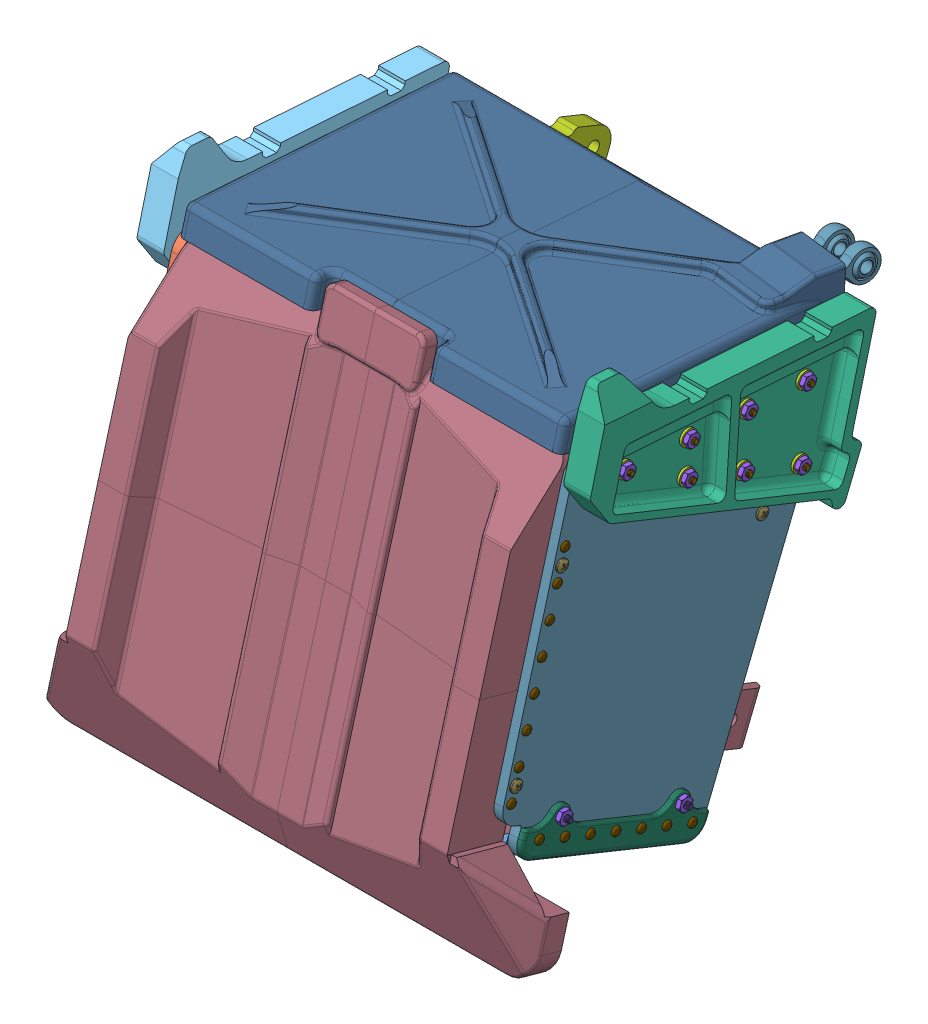
SolidWorks assembly Parachute Container, configuration Default. Lengths in mm.
Overall size (347.79 389.1 362.5).
212 component instances, 33 part files, 129 mates.
Components (placement in the parent):
- Lower Parachute Container Base-1: Lower Parachute Container Base [Default] at (52.975 915.6122 -565.1886) x (0 0.374607 0.927184) z (0 0.927184 -0.374607) size (142.76 271.37 12.7)
- FWD Parachute Container Support-1: FWD Parachute Container Support [Default] at (135.9507 904.2567 -654.4269) x (-1 0 0) z (0 0.264079 0.964501) size (246.23 199.77 12.7)
- Top Parachute Container Base-1: Top Parachute Container Base [Default] at (135.8167 1095.6538 -582.4469) x (0 -0.074087 -0.997252) z (0 0.997252 -0.074087) size (174.02 271.37 12.7)
- Side Parachute Container Support-1: Side Parachute Container Support [Default] at (135.8167 927.3874 -569.9461) x (0 0.374607 0.927184) z (1 0 0) size (157.08 248.25 12.7)
- Aft Parachute Container Support-1: Aft Parachute Container Support [Default] at (52.975 927.3874 -569.9461) x (0 0.374607 0.927184) z (0 0.927184 -0.374607) size (12.7 271.37 248.25)
- LH Canopy Breaker-1: LH Canopy Breaker [Default] at (142.1667 927.3874 -569.9461) x (0 0.374607 0.927184) z (1 0 0) size (208.18 112.77 19.61)
- 98023A113 - WASHER, #8, STEEL, ZINC-1: 98023A113 - WASHER, #8, STEEL, ZINC [98023A113] at (148.5167 1083.7351 -810.3922) x (0 0.665424 0.746466) z (0 0.746466 -0.665424) size (11.11 1.65 11.11)
- 90480A009 - NUT, 8-32, STEEL-1: 90480A009 - NUT, 8-32, STEEL [90480A009] at (151.7552 1083.7351 -810.3922) x (0 -0.999736 0.022959) z (0 -0.022959 -0.999736) size (8.73 3.79 10.08)
- 90275A196 - FHS, 82 CSK, 8-32 X .625, STEEL, ZINC-1: 90275A196 - FHS, 82 CSK, 8-32 X .625, STEEL, ZINC [90275A196] at (141.8239 1083.7351 -810.3922) x (0 -0.799552 -0.600598) z (-1 0 0) size (7.86 7.92 16.2)
- Parachute Container Lid-1: Parachute Container Lid [A] at (135.9507 1108.3189 -583.3878) x (0 -0.074087 -0.997252) z (0 0.997252 -0.074087) size (205.47 137.55 40.32)
- Parachute Container Lid-2: Parachute Container Lid [B] at (135.9507 1108.3189 -583.3878) x (0 -0.074087 -0.997252) z (0 0.997252 -0.074087) size (196.05 135.68 33.77)
- 98023A113 - WASHER, #8, STEEL, ZINC-2: 98023A113 - WASHER, #8, STEEL, ZINC [98023A113] at (110.5507 1073.4536 -858.9887) x (-0.704374 0.052589 0.707878) z (-0.709829 -0.052185 -0.702438) size (11.11 1.65 11.11)
- 93365A140 - INSERT, 8-32, BRASS, FOR PLASTICS-1: 93365A140 - INSERT, 8-32, BRASS, FOR PLASTICS [93365A140] at (110.5507 1087.7651 -860.052) x (0.28611 -0.07099 -0.955563) z (-0.958197 -0.021197 -0.285324) size (6.35 5.19 6.35)
- 91249A197 - PHS, 8-32 x .750, 18-8, BLACK-OXIDE-1: 91249A197 - PHS, 8-32 x .750, 18-8, BLACK-OXIDE [91249A197] at (110.5507 1092.4512 -860.4001) x (0.880302 -0.035148 -0.47311) z (0 -0.997252 0.074087) size (8.18 8.18 22.03)
- SJU-17 Headrest v2-1: SJU-17 Headrest v2 [A] at (25.6344 1058.4473 -689.3362) x (1 0 0) z (0 -0.964501 0.264079) size (135.53 40.86 153.72)
- SJU-17 Headrest v2-2: SJU-17 Headrest v2 [D] at (25.6344 1058.4473 -689.3362) x (1 0 0) z (0 -0.964501 0.264079) size (135.53 40.86 153.72)
- SJU-17 Headrest v2-3: SJU-17 Headrest v2 [C] at (25.6344 1058.4473 -689.3362) x (1 0 0) z (0 -0.964501 0.264079) size (173.89 57.45 153.72)
- SJU-17 Headrest v2-4: SJU-17 Headrest v2 [B] at (25.6344 1058.4473 -689.3362) x (1 0 0) z (0 -0.964501 0.264079) size (173.89 57.45 153.72)
- 98023A113 - WASHER, #8, STEEL, ZINC-3: 98023A113 - WASHER, #8, STEEL, ZINC [98023A113] at (110.2446 1068.5152 -714.2799) x (0.900625 0.41917 -0.114768) z (0.434597 -0.868654 0.237836) size (11.11 1.65 11.11)
- 93365A140 - INSERT, 8-32, BRASS, FOR PLASTICS-2: 93365A140 - INSERT, 8-32, BRASS, FOR PLASTICS [93365A140] at (110.2446 1072.305 -700.4383) x (-0.589007 -0.77944 0.21341) z (0.808128 -0.568098 0.155545) size (6.35 5.19 6.35)
- 91249A197 - PHS, 8-32 x .750, 18-8, BLACK-OXIDE-2: 91249A197 - PHS, 8-32 x .750, 18-8, BLACK-OXIDE [91249A197] at (110.2446 1073.5459 -695.9061) x (-0.988068 -0.14855 0.040673) z (0 -0.264079 -0.964501) size (8.18 8.18 22.03)
- Outside Parachute Container Skin-1: Outside Parachute Container Skin [Default] at (135.8167 927.3874 -569.9461) x (0 0.374607 0.927184) z (1 0 0) size (182.93 279.31 6.35)
- Lower Parachute Container Skin Trim-1: Lower Parachute Container Skin Trim [Default] at (142.1667 0 0) x (0 0 -1) z (1 0 0) size (134.99 73.21 3.28)
- 91249A197 - PHS, 8-32 x .750, 18-8, BLACK-OXIDE-3: 91249A197 - PHS, 8-32 x .750, 18-8, BLACK-OXIDE [91249A197] at (123.1167 1007.3681 -828.0549) x (0 0.923939 0.382539) z (1 0 0) size (8.18 8.18 22.03)
- 92105A660 - INSERT, 8-32, SELF TAPPING, FOR SOFTWOOD-1: 92105A660 - INSERT, 8-32, SELF TAPPING, FOR SOFTWOOD [92105A660] at (135.8167 1007.3681 -828.0549) x (0 -0.986773 0.162111) z (0 0.162111 0.986773) size (7.16 10.23 7.14)
- 90480A009 - NUT, 8-32, STEEL-2: 90480A009 - NUT, 8-32, STEEL [90480A009] at (146.9292 860.255 -768.6173) x (0 0.987351 0.158553) z (0 -0.158553 0.987351) size (8.73 3.79 10.08)
- 92105A660 - INSERT, 8-32, SELF TAPPING, FOR SOFTWOOD-2: 92105A660 - INSERT, 8-32, SELF TAPPING, FOR SOFTWOOD [92105A660] at (123.1167 860.255 -768.6173) x (0 -0.526625 0.850097) z (0 -0.850097 -0.526625) size (7.16 10.23 7.14)
- 90480A009 - NUT, 8-32, STEEL-3: 90480A009 - NUT, 8-32, STEEL [90480A009] at (121.5292 860.255 -768.6173) x (0 0.987351 0.158553) z (0 -0.158553 0.987351) size (8.73 3.79 10.08)
- 90272A201 - PHS, 8-32 x 1.250, STEEL, ZINC-1: 90272A201 - PHS, 8-32 x 1.250, STEEL, ZINC [90272A201] at (151.6917 860.255 -768.6173) x (0 -0.158553 0.987351) z (-1 0 0) size (8.18 8.18 34.79)
- 90272A201 - PHS, 8-32 x 1.250, STEEL, ZINC-2: 90272A201 - PHS, 8-32 x 1.250, STEEL, ZINC [90272A201] at (151.6917 894.7022 -683.3576) x (0 0 1) z (-1 0 0) size (8.18 8.18 34.79)
- 90480A009 - NUT, 8-32, STEEL-4: 90480A009 - NUT, 8-32, STEEL [90480A009] at (121.5292 894.7022 -683.3576) x (0 1 0) z (0 0 1) size (8.73 3.79 10.08)
- 92105A660 - INSERT, 8-32, SELF TAPPING, FOR SOFTWOOD-3: 92105A660 - INSERT, 8-32, SELF TAPPING, FOR SOFTWOOD [92105A660] at (123.1167 894.7022 -683.3576) x (0 -0.385179 0.922842) z (0 -0.922842 -0.385179) size (7.16 10.23 7.14)
- 90480A009 - NUT, 8-32, STEEL-5: 90480A009 - NUT, 8-32, STEEL [90480A009] at (146.9292 894.7022 -683.3576) x (0 1 0) z (0 0 1) size (8.73 3.79 10.08)
- 91249A197 - PHS, 8-32 x .750, 18-8, BLACK-OXIDE-4: 91249A197 - PHS, 8-32 x .750, 18-8, BLACK-OXIDE [91249A197] at (123.1167 926.9171 -652.9942) x (0 0.851599 0.524194) z (1 0 0) size (8.18 8.18 22.03)
- 93365A140 - INSERT, 8-32, BRASS, FOR PLASTICS-3: 93365A140 - INSERT, 8-32, BRASS, FOR PLASTICS [93365A140] at (135.674 926.9158 -652.9941) x (0.000012 -0.033074 0.999453) z (-0.0002 0.999453 0.033074) size (6.35 5.19 6.35)
- 91249A197 - PHS, 8-32 x .750, 18-8, BLACK-OXIDE-5: 91249A197 - PHS, 8-32 x .750, 18-8, BLACK-OXIDE [91249A197] at (123.1167 1046.3464 -685.6938) x (0 0.923939 0.382539) z (1 0 0) size (8.18 8.18 22.03)
- 93365A140 - INSERT, 8-32, BRASS, FOR PLASTICS-4: 93365A140 - INSERT, 8-32, BRASS, FOR PLASTICS [93365A140] at (135.6498 1046.3451 -685.6937) x (-0.00002 0.125847 0.99205) z (-0.0002 0.99205 -0.125847) size (6.35 5.19 6.35)
- 91654A144 - SCREW NAIL, DOMED, .14 X .25 SHANK X .25 HD DIA, 18-8-1: 91654A144 - SCREW NAIL, DOMED, .14 X .25 SHANK X .25 HD DIA, 18-8 [Default] at (138.9917 888.1671 -667.0198) x (0 -0.807538 -0.589816) z (0 -0.589816 0.807538) size (6.35 7.94 6.35)
- 91654A144 - SCREW NAIL, DOMED, .14 X .25 SHANK X .25 HD DIA, 18-8-2: 91654A144 - SCREW NAIL, DOMED, .14 X .25 SHANK X .25 HD DIA, 18-8 [Default] at (135.8167 1056.2989 -688.4187) x (0 -0.89084 -0.454318) z (0 -0.454318 0.89084) size (6.35 7.94 6.35)
- 90252A11X - FHS, 82 DEG, #8, BLK, STEEL, FOR MDF-1: 90252A11X - FHS, 82 DEG, #8, BLK, STEEL, FOR MDF [90252A112] at (129.4667 1095.7252 -746.2449) x (0.473301 0.065264 0.87848) z (-0.880901 0.035066 0.472) size (8.43 25 8.43)
- 90252A11X - FHS, 82 DEG, #8, BLK, STEEL, FOR MDF-2: 90252A11X - FHS, 82 DEG, #8, BLK, STEEL, FOR MDF [90252A112] at (135.3233 1065.2704 -707.1666) x (0 -0.406737 0.913545) z (0 0.913545 0.406737) size (8.43 25 8.43)
- 90252A11X - FHS, 82 DEG, #8, BLK, STEEL, FOR MDF-3: 90252A11X - FHS, 82 DEG, #8, BLK, STEEL, FOR MDF [90252A112] at (129.4667 1050.3798 -872.2953) x (-0.694658 0.66696 -0.269469) z (-0.71934 -0.644076 0.260224) size (8.43 25 8.43)
- 90252A11X - FHS, 82 DEG, #8, BLK, STEEL, FOR MDF-4: 90252A11X - FHS, 82 DEG, #8, BLK, STEEL, FOR MDF [90252A112] at (129.4667 869.7131 -680.11) x (-0.694658 -0.269469 -0.66696) z (-0.71934 0.260224 0.644076) size (8.43 25 8.43)
- Right Outside Parachute Container Skin-2: Right Outside Parachute Container Skin [Default] at (-135.8167 927.3874 -569.9461) x (0 0.374607 0.927184) z (1 0 0) size (182.93 279.31 6.35)
- Right Lower Parachute Container Skin Trim-3: Right Lower Parachute Container Skin Trim [Default] at (-142.1667 0 0) x (0 0 -1) z (1 0 0) size (134.99 73.21 3.28)
- Right Side Parachute Container Support-2: Right Side Parachute Container Support [Default] at (-135.8167 927.3874 -569.9461) x (0 0.374607 0.927184) z (1 0 0) size (157.08 248.25 12.7)
- RH Canopy Breaker-2: RH Canopy Breaker [Default] at (-142.1667 927.3874 -569.9461) x (0 0.374607 0.927184) z (1 0 0) size (208.18 112.77 19.61)
- 90252A11X - FHS, 82 DEG, #8, BLK, STEEL, FOR MDF-5: 90252A11X - FHS, 82 DEG, #8, BLK, STEEL, FOR MDF [90252A112] at (-129.2574 1088.4631 -843.9962) x (0.473301 0.065264 0.87848) z (-0.880901 0.035066 0.472) size (8.43 25 8.43)
- 90252A11X - FHS, 82 DEG, #8, BLK, STEEL, FOR MDF-6: 90252A11X - FHS, 82 DEG, #8, BLK, STEEL, FOR MDF [90252A112] at (-129.4082 1095.7104 -746.4439) x (0.473301 0.065264 0.87848) z (-0.880901 0.035066 0.472) size (8.43 25 8.43)
- 90252A11X - FHS, 82 DEG, #8, BLK, STEEL, FOR MDF-7: 90252A11X - FHS, 82 DEG, #8, BLK, STEEL, FOR MDF [90252A112] at (129.4667 1088.4779 -843.7973) x (0.473301 0.065264 0.87848) z (-0.880901 0.035066 0.472) size (8.43 25 8.43)
- 90252A11X - FHS, 82 DEG, #8, BLK, STEEL, FOR MDF-8: 90252A11X - FHS, 82 DEG, #8, BLK, STEEL, FOR MDF [90252A112] at (135.3233 944.6031 -674.128) x (0 -0.406737 0.913545) z (0 0.913545 0.406737) size (8.43 25 8.43)
- 90252A11X - FHS, 82 DEG, #8, BLK, STEEL, FOR MDF-9: 90252A11X - FHS, 82 DEG, #8, BLK, STEEL, FOR MDF [90252A112] at (-135.3233 1065.2704 -707.1666) x (0 -0.406737 0.913545) z (0 -0.913545 -0.406737) size (8.43 25 8.43)
- 90252A11X - FHS, 82 DEG, #8, BLK, STEEL, FOR MDF-10: 90252A11X - FHS, 82 DEG, #8, BLK, STEEL, FOR MDF [90252A112] at (-135.3233 944.6031 -674.128) x (0 -0.406737 0.913545) z (0 -0.913545 -0.406737) size (8.43 25 8.43)
- 90252A11X - FHS, 82 DEG, #8, BLK, STEEL, FOR MDF-11: 90252A11X - FHS, 82 DEG, #8, BLK, STEEL, FOR MDF [90252A112] at (-129.1988 1050.3798 -872.2953) x (-0.694658 0.66696 -0.269469) z (-0.71934 -0.644076 0.260224) size (8.43 25 8.43)
- 90252A11X - FHS, 82 DEG, #8, BLK, STEEL, FOR MDF-12: 90252A11X - FHS, 82 DEG, #8, BLK, STEEL, FOR MDF [90252A112] at (-129.1988 890.8578 -807.8443) x (-0.694658 0.66696 -0.269469) z (-0.71934 -0.644076 0.260224) size (8.43 25 8.43)
- 90252A11X - FHS, 82 DEG, #8, BLK, STEEL, FOR MDF-13: 90252A11X - FHS, 82 DEG, #8, BLK, STEEL, FOR MDF [90252A112] at (129.4667 890.8578 -807.8443) x (-0.694658 0.66696 -0.269469) z (-0.71934 -0.644076 0.260224) size (8.43 25 8.43)
- 90252A11X - FHS, 82 DEG, #8, BLK, STEEL, FOR MDF-14: 90252A11X - FHS, 82 DEG, #8, BLK, STEEL, FOR MDF [90252A112] at (-129.1988 840.0234 -753.5946) x (-0.694658 -0.269469 -0.66696) z (-0.71934 0.260224 0.644076) size (8.43 25 8.43)
- 90252A11X - FHS, 82 DEG, #8, BLK, STEEL, FOR MDF-15: 90252A11X - FHS, 82 DEG, #8, BLK, STEEL, FOR MDF [90252A112] at (-129.1988 869.7131 -680.11) x (-0.694658 -0.269469 -0.66696) z (-0.71934 0.260224 0.644076) size (8.43 25 8.43)
- 90252A11X - FHS, 82 DEG, #8, BLK, STEEL, FOR MDF-16: 90252A11X - FHS, 82 DEG, #8, BLK, STEEL, FOR MDF [90252A112] at (-110.1488 830.5084 -777.145) x (-0.694658 -0.269469 -0.66696) z (-0.71934 0.260224 0.644076) size (8.43 25 8.43)
- 90252A11X - FHS, 82 DEG, #8, BLK, STEEL, FOR MDF-17: 90252A11X - FHS, 82 DEG, #8, BLK, STEEL, FOR MDF [90252A112] at (0.134 830.5084 -777.145) x (-0.694658 -0.269469 -0.66696) z (-0.71934 0.260224 0.644076) size (8.43 25 8.43)
- 90252A11X - FHS, 82 DEG, #8, BLK, STEEL, FOR MDF-18: 90252A11X - FHS, 82 DEG, #8, BLK, STEEL, FOR MDF [90252A112] at (110.4167 830.5084 -777.145) x (-0.694658 -0.269469 -0.66696) z (-0.71934 0.260224 0.644076) size (8.43 25 8.43)
- 90252A11X - FHS, 82 DEG, #8, BLK, STEEL, FOR MDF-19: 90252A11X - FHS, 82 DEG, #8, BLK, STEEL, FOR MDF [90252A112] at (129.4667 840.0234 -753.5946) x (-0.694658 -0.269469 -0.66696) z (-0.71934 0.260224 0.644076) size (8.43 25 8.43)
- 93365A140 - INSERT, 8-32, BRASS, FOR PLASTICS-5: 93365A140 - INSERT, 8-32, BRASS, FOR PLASTICS [93365A140] at (110.2446 908.8361 -655.6807) x (-0.589007 -0.77944 0.21341) z (0.808128 -0.568098 0.155545) size (6.35 5.19 6.35)
- 93365A140 - INSERT, 8-32, BRASS, FOR PLASTICS-6: 93365A140 - INSERT, 8-32, BRASS, FOR PLASTICS [93365A140] at (19.184 956.3053 -668.6777) x (-0.589007 -0.77944 0.21341) z (0.808128 -0.568098 0.155545) size (6.35 5.19 6.35)
- 93365A140 - INSERT, 8-32, BRASS, FOR PLASTICS-7: 93365A140 - INSERT, 8-32, BRASS, FOR PLASTICS [93365A140] at (-109.9766 908.8361 -655.6807) x (-0.589007 -0.77944 0.21341) z (0.808128 -0.568098 0.155545) size (6.35 5.19 6.35)
- 93365A140 - INSERT, 8-32, BRASS, FOR PLASTICS-8: 93365A140 - INSERT, 8-32, BRASS, FOR PLASTICS [93365A140] at (-18.916 956.3053 -668.6777) x (-0.589007 -0.77944 0.21341) z (0.808128 -0.568098 0.155545) size (6.35 5.19 6.35)
- 93365A140 - INSERT, 8-32, BRASS, FOR PLASTICS-9: 93365A140 - INSERT, 8-32, BRASS, FOR PLASTICS [93365A140] at (-109.9766 1072.305 -700.4383) x (-0.589007 -0.77944 0.21341) z (0.808128 -0.568098 0.155545) size (6.35 5.19 6.35)
- 93365A140 - INSERT, 8-32, BRASS, FOR PLASTICS-10: 93365A140 - INSERT, 8-32, BRASS, FOR PLASTICS [93365A140] at (-18.916 993.0528 -678.7391) x (-0.589007 -0.77944 0.21341) z (0.808128 -0.568098 0.155545) size (6.35 5.19 6.35)
- 93365A140 - INSERT, 8-32, BRASS, FOR PLASTICS-11: 93365A140 - INSERT, 8-32, BRASS, FOR PLASTICS [93365A140] at (19.184 993.0528 -678.7391) x (-0.589007 -0.77944 0.21341) z (0.808128 -0.568098 0.155545) size (6.35 5.19 6.35)
- 98023A113 - WASHER, #8, STEEL, ZINC-4: 98023A113 - WASHER, #8, STEEL, ZINC [98023A113] at (110.2446 905.0463 -669.5223) x (0.900625 0.41917 -0.114768) z (0.434597 -0.868654 0.237836) size (11.11 1.65 11.11)
- 98023A113 - WASHER, #8, STEEL, ZINC-5: 98023A113 - WASHER, #8, STEEL, ZINC [98023A113] at (19.184 952.5155 -682.5193) x (0.900625 0.41917 -0.114768) z (0.434597 -0.868654 0.237836) size (11.11 1.65 11.11)
- 98023A113 - WASHER, #8, STEEL, ZINC-6: 98023A113 - WASHER, #8, STEEL, ZINC [98023A113] at (-109.9766 905.0463 -669.5223) x (0.900625 0.41917 -0.114768) z (0.434597 -0.868654 0.237836) size (11.11 1.65 11.11)
- 98023A113 - WASHER, #8, STEEL, ZINC-7: 98023A113 - WASHER, #8, STEEL, ZINC [98023A113] at (-18.916 952.5155 -682.5193) x (0.900625 0.41917 -0.114768) z (0.434597 -0.868654 0.237836) size (11.11 1.65 11.11)
- 98023A113 - WASHER, #8, STEEL, ZINC-8: 98023A113 - WASHER, #8, STEEL, ZINC [98023A113] at (-109.9766 1068.5152 -714.2799) x (0.900625 0.41917 -0.114768) z (0.434597 -0.868654 0.237836) size (11.11 1.65 11.11)
- 98023A113 - WASHER, #8, STEEL, ZINC-9: 98023A113 - WASHER, #8, STEEL, ZINC [98023A113] at (-18.916 989.263 -692.5807) x (0.900625 0.41917 -0.114768) z (0.434597 -0.868654 0.237836) size (11.11 1.65 11.11)
- 98023A113 - WASHER, #8, STEEL, ZINC-10: 98023A113 - WASHER, #8, STEEL, ZINC [98023A113] at (19.184 989.263 -692.5807) x (0.900625 0.41917 -0.114768) z (0.434597 -0.868654 0.237836) size (11.11 1.65 11.11)
- 91249A197 - PHS, 8-32 x .750, 18-8, BLACK-OXIDE-6: 91249A197 - PHS, 8-32 x .750, 18-8, BLACK-OXIDE [91249A197] at (110.2446 910.077 -651.1485) x (-0.988068 -0.14855 0.040673) z (0 -0.264079 -0.964501) size (8.18 8.18 22.03)
- 91249A197 - PHS, 8-32 x .750, 18-8, BLACK-OXIDE-7: 91249A197 - PHS, 8-32 x .750, 18-8, BLACK-OXIDE [91249A197] at (19.184 957.5462 -664.1455) x (-0.988068 -0.14855 0.040673) z (0 -0.264079 -0.964501) size (8.18 8.18 22.03)
- 91249A197 - PHS, 8-32 x .750, 18-8, BLACK-OXIDE-8: 91249A197 - PHS, 8-32 x .750, 18-8, BLACK-OXIDE [91249A197] at (-109.9766 910.077 -651.1485) x (-0.988068 -0.14855 0.040673) z (0 -0.264079 -0.964501) size (8.18 8.18 22.03)
- 91249A197 - PHS, 8-32 x .750, 18-8, BLACK-OXIDE-9: 91249A197 - PHS, 8-32 x .750, 18-8, BLACK-OXIDE [91249A197] at (-18.916 957.5462 -664.1455) x (-0.988068 -0.14855 0.040673) z (0 -0.264079 -0.964501) size (8.18 8.18 22.03)
- 91249A197 - PHS, 8-32 x .750, 18-8, BLACK-OXIDE-10: 91249A197 - PHS, 8-32 x .750, 18-8, BLACK-OXIDE [91249A197] at (-109.9766 1073.5459 -695.9061) x (-0.988068 -0.14855 0.040673) z (0 -0.264079 -0.964501) size (8.18 8.18 22.03)
- 91249A197 - PHS, 8-32 x .750, 18-8, BLACK-OXIDE-11: 91249A197 - PHS, 8-32 x .750, 18-8, BLACK-OXIDE [91249A197] at (-18.916 994.2937 -674.207) x (-0.988068 -0.14855 0.040673) z (0 -0.264079 -0.964501) size (8.18 8.18 22.03)
- 91249A197 - PHS, 8-32 x .750, 18-8, BLACK-OXIDE-12: 91249A197 - PHS, 8-32 x .750, 18-8, BLACK-OXIDE [91249A197] at (19.184 994.2937 -674.207) x (-0.988068 -0.14855 0.040673) z (0 -0.264079 -0.964501) size (8.18 8.18 22.03)
- 93365A140 - INSERT, 8-32, BRASS, FOR PLASTICS-12: 93365A140 - INSERT, 8-32, BRASS, FOR PLASTICS [93365A140] at (110.5507 1097.1582 -733.6163) x (0.28611 -0.07099 -0.955563) z (-0.958197 -0.021197 -0.285324) size (6.35 5.19 6.35)
- 93365A140 - INSERT, 8-32, BRASS, FOR PLASTICS-13: 93365A140 - INSERT, 8-32, BRASS, FOR PLASTICS [93365A140] at (-110.0148 1087.7651 -860.052) x (0.28611 -0.07099 -0.955563) z (-0.958197 -0.021197 -0.285324) size (6.35 5.19 6.35)
- 93365A140 - INSERT, 8-32, BRASS, FOR PLASTICS-14: 93365A140 - INSERT, 8-32, BRASS, FOR PLASTICS [93365A140] at (25.668 1092.6381 -794.4594) x (0.28611 -0.07099 -0.955563) z (-0.958197 -0.021197 -0.285324) size (6.35 5.19 6.35)
- 93365A140 - INSERT, 8-32, BRASS, FOR PLASTICS-15: 93365A140 - INSERT, 8-32, BRASS, FOR PLASTICS [93365A140] at (-110.0148 1097.1582 -733.6163) x (0.28611 -0.07099 -0.955563) z (-0.958197 -0.021197 -0.285324) size (6.35 5.19 6.35)
- 93365A140 - INSERT, 8-32, BRASS, FOR PLASTICS-16: 93365A140 - INSERT, 8-32, BRASS, FOR PLASTICS [93365A140] at (-25.132 1092.6381 -794.4594) x (0.28611 -0.07099 -0.955563) z (-0.958197 -0.021197 -0.285324) size (6.35 5.19 6.35)
- 91249A197 - PHS, 8-32 x .750, 18-8, BLACK-OXIDE-13: 91249A197 - PHS, 8-32 x .750, 18-8, BLACK-OXIDE [91249A197] at (110.5507 1101.8443 -733.9644) x (0.880302 -0.035148 -0.47311) z (0 -0.997252 0.074087) size (8.18 8.18 22.03)
- 91249A197 - PHS, 8-32 x .750, 18-8, BLACK-OXIDE-14: 91249A197 - PHS, 8-32 x .750, 18-8, BLACK-OXIDE [91249A197] at (-110.0148 1092.4512 -860.4001) x (0.880302 -0.035148 -0.47311) z (0 -0.997252 0.074087) size (8.18 8.18 22.03)
- 91249A197 - PHS, 8-32 x .750, 18-8, BLACK-OXIDE-15: 91249A197 - PHS, 8-32 x .750, 18-8, BLACK-OXIDE [91249A197] at (25.668 1097.3242 -794.8075) x (0.880302 -0.035148 -0.47311) z (0 -0.997252 0.074087) size (8.18 8.18 22.03)
- 91249A197 - PHS, 8-32 x .750, 18-8, BLACK-OXIDE-16: 91249A197 - PHS, 8-32 x .750, 18-8, BLACK-OXIDE [91249A197] at (-110.0148 1101.8443 -733.9644) x (0.880302 -0.035148 -0.47311) z (0 -0.997252 0.074087) size (8.18 8.18 22.03)
- 91249A197 - PHS, 8-32 x .750, 18-8, BLACK-OXIDE-17: 91249A197 - PHS, 8-32 x .750, 18-8, BLACK-OXIDE [91249A197] at (-25.132 1097.3242 -794.8075) x (0.880302 -0.035148 -0.47311) z (0 -0.997252 0.074087) size (8.18 8.18 22.03)
- 98023A113 - WASHER, #8, STEEL, ZINC-11: 98023A113 - WASHER, #8, STEEL, ZINC [98023A113] at (110.5507 1082.8467 -732.5531) x (-0.704374 0.052589 0.707878) z (-0.709829 -0.052185 -0.702438) size (11.11 1.65 11.11)
- 98023A113 - WASHER, #8, STEEL, ZINC-12: 98023A113 - WASHER, #8, STEEL, ZINC [98023A113] at (-110.0148 1073.4536 -858.9887) x (-0.704374 0.052589 0.707878) z (-0.709829 -0.052185 -0.702438) size (11.11 1.65 11.11)
- 98023A113 - WASHER, #8, STEEL, ZINC-13: 98023A113 - WASHER, #8, STEEL, ZINC [98023A113] at (25.668 1078.3265 -793.3962) x (-0.704374 0.052589 0.707878) z (-0.709829 -0.052185 -0.702438) size (11.11 1.65 11.11)
- 98023A113 - WASHER, #8, STEEL, ZINC-14: 98023A113 - WASHER, #8, STEEL, ZINC [98023A113] at (-110.0148 1082.8467 -732.5531) x (-0.704374 0.052589 0.707878) z (-0.709829 -0.052185 -0.702438) size (11.11 1.65 11.11)
- 98023A113 - WASHER, #8, STEEL, ZINC-15: 98023A113 - WASHER, #8, STEEL, ZINC [98023A113] at (-25.132 1078.3265 -793.3962) x (-0.704374 0.052589 0.707878) z (-0.709829 -0.052185 -0.702438) size (11.11 1.65 11.11)
- 90275A196 - FHS, 82 CSK, 8-32 X .625, STEEL, ZINC-2: 90275A196 - FHS, 82 CSK, 8-32 X .625, STEEL, ZINC [90275A196] at (141.8239 1089.774 -723.628) x (0 -0.799552 -0.600598) z (-1 0 0) size (7.86 7.92 16.2)
- 90275A196 - FHS, 82 CSK, 8-32 X .625, STEEL, ZINC-3: 90275A196 - FHS, 82 CSK, 8-32 X .625, STEEL, ZINC [90275A196] at (141.8239 1086.6009 -769.2168) x (0 -0.799552 -0.600598) z (-1 0 0) size (7.86 7.92 16.2)
- 90275A196 - FHS, 82 CSK, 8-32 X .625, STEEL, ZINC-4: 90275A196 - FHS, 82 CSK, 8-32 X .625, STEEL, ZINC [90275A196] at (141.8239 1063.3673 -767.5997) x (0 -0.799552 -0.600598) z (-1 0 0) size (7.86 7.92 16.2)
- 90275A196 - FHS, 82 CSK, 8-32 X .625, STEEL, ZINC-5: 90275A196 - FHS, 82 CSK, 8-32 X .625, STEEL, ZINC [90275A196] at (141.8239 1047.2333 -807.8516) x (0 -0.799552 -0.600598) z (-1 0 0) size (7.86 7.92 16.2)
- 90275A196 - FHS, 82 CSK, 8-32 X .625, STEEL, ZINC-6: 90275A196 - FHS, 82 CSK, 8-32 X .625, STEEL, ZINC [90275A196] at (141.8239 1030.9554 -848.4627) x (0 -0.799552 -0.600598) z (-1 0 0) size (7.86 7.92 16.2)
- 90275A196 - FHS, 82 CSK, 8-32 X .625, STEEL, ZINC-7: 90275A196 - FHS, 82 CSK, 8-32 X .625, STEEL, ZINC [90275A196] at (141.8239 1080.8436 -851.935) x (0 -0.799552 -0.600598) z (-1 0 0) size (7.86 7.92 16.2)
- 90480A009 - NUT, 8-32, STEEL-6: 90480A009 - NUT, 8-32, STEEL [90480A009] at (151.7552 1089.774 -723.628) x (0 -0.999736 0.022959) z (0 -0.022959 -0.999736) size (8.73 3.79 10.08)
- 90480A009 - NUT, 8-32, STEEL-7: 90480A009 - NUT, 8-32, STEEL [90480A009] at (151.7552 1086.6009 -769.2168) x (0 -0.999736 0.022959) z (0 -0.022959 -0.999736) size (8.73 3.79 10.08)
- 90480A009 - NUT, 8-32, STEEL-8: 90480A009 - NUT, 8-32, STEEL [90480A009] at (151.7552 1063.3673 -767.5997) x (0 -0.999736 0.022959) z (0 -0.022959 -0.999736) size (8.73 3.79 10.08)
- 90480A009 - NUT, 8-32, STEEL-9: 90480A009 - NUT, 8-32, STEEL [90480A009] at (151.7552 1047.2333 -807.8516) x (0 -0.999736 0.022959) z (0 -0.022959 -0.999736) size (8.73 3.79 10.08)
- 90480A009 - NUT, 8-32, STEEL-10: 90480A009 - NUT, 8-32, STEEL [90480A009] at (151.7552 1030.9554 -848.4627) x (0 -0.999736 0.022959) z (0 -0.022959 -0.999736) size (8.73 3.79 10.08)
- 90480A009 - NUT, 8-32, STEEL-11: 90480A009 - NUT, 8-32, STEEL [90480A009] at (151.7552 1080.8436 -851.935) x (0 -0.999736 0.022959) z (0 -0.022959 -0.999736) size (8.73 3.79 10.08)
- 98023A113 - WASHER, #8, STEEL, ZINC-16: 98023A113 - WASHER, #8, STEEL, ZINC [98023A113] at (148.5167 1089.774 -723.628) x (0 0.665424 0.746466) z (0 0.746466 -0.665424) size (11.11 1.65 11.11)
- 98023A113 - WASHER, #8, STEEL, ZINC-17: 98023A113 - WASHER, #8, STEEL, ZINC [98023A113] at (148.5167 1086.6009 -769.2168) x (0 0.665424 0.746466) z (0 0.746466 -0.665424) size (11.11 1.65 11.11)
- 98023A113 - WASHER, #8, STEEL, ZINC-18: 98023A113 - WASHER, #8, STEEL, ZINC [98023A113] at (148.5167 1063.3673 -767.5997) x (0 0.665424 0.746466) z (0 0.746466 -0.665424) size (11.11 1.65 11.11)
- 98023A113 - WASHER, #8, STEEL, ZINC-19: 98023A113 - WASHER, #8, STEEL, ZINC [98023A113] at (148.5167 1047.2333 -807.8516) x (0 0.665424 0.746466) z (0 0.746466 -0.665424) size (11.11 1.65 11.11)
- 98023A113 - WASHER, #8, STEEL, ZINC-20: 98023A113 - WASHER, #8, STEEL, ZINC [98023A113] at (148.5167 1030.9554 -848.4627) x (0 0.665424 0.746466) z (0 0.746466 -0.665424) size (11.11 1.65 11.11)
- 98023A113 - WASHER, #8, STEEL, ZINC-21: 98023A113 - WASHER, #8, STEEL, ZINC [98023A113] at (148.5167 1080.8436 -851.935) x (0 0.665424 0.746466) z (0 0.746466 -0.665424) size (11.11 1.65 11.11)
- 91654A144 - SCREW NAIL, DOMED, .14 X .25 SHANK X .25 HD DIA, 18-8-3: 91654A144 - SCREW NAIL, DOMED, .14 X .25 SHANK X .25 HD DIA, 18-8 [Default] at (135.8167 916.9647 -650.2692) x (0 -0.89084 -0.454318) z (0 -0.454318 0.89084) size (6.35 7.94 6.35)
- 91654A144 - SCREW NAIL, DOMED, .14 X .25 SHANK X .25 HD DIA, 18-8-4: 91654A144 - SCREW NAIL, DOMED, .14 X .25 SHANK X .25 HD DIA, 18-8 [Default] at (135.8167 1036.394 -682.9688) x (0 -0.89084 -0.454318) z (0 -0.454318 0.89084) size (6.35 7.94 6.35)
- 91654A144 - SCREW NAIL, DOMED, .14 X .25 SHANK X .25 HD DIA, 18-8-5: 91654A144 - SCREW NAIL, DOMED, .14 X .25 SHANK X .25 HD DIA, 18-8 [Default] at (135.8167 1016.4891 -677.5189) x (0 -0.89084 -0.454318) z (0 -0.454318 0.89084) size (6.35 7.94 6.35)
- 91654A144 - SCREW NAIL, DOMED, .14 X .25 SHANK X .25 HD DIA, 18-8-6: 91654A144 - SCREW NAIL, DOMED, .14 X .25 SHANK X .25 HD DIA, 18-8 [Default] at (135.8167 996.5842 -672.0689) x (0 -0.89084 -0.454318) z (0 -0.454318 0.89084) size (6.35 7.94 6.35)
- 91654A144 - SCREW NAIL, DOMED, .14 X .25 SHANK X .25 HD DIA, 18-8-7: 91654A144 - SCREW NAIL, DOMED, .14 X .25 SHANK X .25 HD DIA, 18-8 [Default] at (135.8167 976.6793 -666.619) x (0 -0.89084 -0.454318) z (0 -0.454318 0.89084) size (6.35 7.94 6.35)
- 91654A144 - SCREW NAIL, DOMED, .14 X .25 SHANK X .25 HD DIA, 18-8-8: 91654A144 - SCREW NAIL, DOMED, .14 X .25 SHANK X .25 HD DIA, 18-8 [Default] at (135.8167 956.7744 -661.1691) x (0 -0.89084 -0.454318) z (0 -0.454318 0.89084) size (6.35 7.94 6.35)
- 91654A144 - SCREW NAIL, DOMED, .14 X .25 SHANK X .25 HD DIA, 18-8-9: 91654A144 - SCREW NAIL, DOMED, .14 X .25 SHANK X .25 HD DIA, 18-8 [Default] at (135.8167 936.8695 -655.7191) x (0 -0.89084 -0.454318) z (0 -0.454318 0.89084) size (6.35 7.94 6.35)
- 91654A144 - SCREW NAIL, DOMED, .14 X .25 SHANK X .25 HD DIA, 18-8-10: 91654A144 - SCREW NAIL, DOMED, .14 X .25 SHANK X .25 HD DIA, 18-8 [Default] at (138.9917 844.2049 -775.8301) x (0 -0.807538 -0.589816) z (0 -0.589816 0.807538) size (6.35 7.94 6.35)
- 91654A144 - SCREW NAIL, DOMED, .14 X .25 SHANK X .25 HD DIA, 18-8-11: 91654A144 - SCREW NAIL, DOMED, .14 X .25 SHANK X .25 HD DIA, 18-8 [Default] at (138.9917 851.5319 -757.695) x (0 -0.807538 -0.589816) z (0 -0.589816 0.807538) size (6.35 7.94 6.35)
- 91654A144 - SCREW NAIL, DOMED, .14 X .25 SHANK X .25 HD DIA, 18-8-12: 91654A144 - SCREW NAIL, DOMED, .14 X .25 SHANK X .25 HD DIA, 18-8 [Default] at (138.9917 858.8589 -739.56) x (0 -0.807538 -0.589816) z (0 -0.589816 0.807538) size (6.35 7.94 6.35)
- 91654A144 - SCREW NAIL, DOMED, .14 X .25 SHANK X .25 HD DIA, 18-8-13: 91654A144 - SCREW NAIL, DOMED, .14 X .25 SHANK X .25 HD DIA, 18-8 [Default] at (138.9917 866.186 -721.4249) x (0 -0.807538 -0.589816) z (0 -0.589816 0.807538) size (6.35 7.94 6.35)
- 91654A144 - SCREW NAIL, DOMED, .14 X .25 SHANK X .25 HD DIA, 18-8-14: 91654A144 - SCREW NAIL, DOMED, .14 X .25 SHANK X .25 HD DIA, 18-8 [Default] at (138.9917 873.513 -703.2899) x (0 -0.807538 -0.589816) z (0 -0.589816 0.807538) size (6.35 7.94 6.35)
- 91654A144 - SCREW NAIL, DOMED, .14 X .25 SHANK X .25 HD DIA, 18-8-15: 91654A144 - SCREW NAIL, DOMED, .14 X .25 SHANK X .25 HD DIA, 18-8 [Default] at (138.9917 880.84 -685.1549) x (0 -0.807538 -0.589816) z (0 -0.589816 0.807538) size (6.35 7.94 6.35)
- 91249A197 - PHS, 8-32 x .750, 18-8, BLACK-OXIDE-18: 91249A197 - PHS, 8-32 x .750, 18-8, BLACK-OXIDE [91249A197] at (-123.1167 1007.3681 -828.0549) x (0 -0.923939 -0.382539) z (-1 0 0) size (8.18 8.18 22.03)
- 93365A140 - INSERT, 8-32, BRASS, FOR PLASTICS-17: 93365A140 - INSERT, 8-32, BRASS, FOR PLASTICS [93365A140] at (-135.6498 1046.3451 -685.6937) x (-0.00002 -0.125847 -0.99205) z (0.0002 0.99205 -0.125847) size (6.35 5.19 6.35)
- 91249A197 - PHS, 8-32 x .750, 18-8, BLACK-OXIDE-19: 91249A197 - PHS, 8-32 x .750, 18-8, BLACK-OXIDE [91249A197] at (-123.1167 1046.3464 -685.6938) x (0 -0.923939 -0.382539) z (-1 0 0) size (8.18 8.18 22.03)
- 93365A140 - INSERT, 8-32, BRASS, FOR PLASTICS-18: 93365A140 - INSERT, 8-32, BRASS, FOR PLASTICS [93365A140] at (-135.674 926.9158 -652.9941) x (0.000012 0.033074 -0.999453) z (0.0002 0.999453 0.033074) size (6.35 5.19 6.35)
- 91249A197 - PHS, 8-32 x .750, 18-8, BLACK-OXIDE-20: 91249A197 - PHS, 8-32 x .750, 18-8, BLACK-OXIDE [91249A197] at (-123.1167 926.9171 -652.9942) x (0 -0.851599 -0.524194) z (-1 0 0) size (8.18 8.18 22.03)
- 90480A009 - NUT, 8-32, STEEL-12: 90480A009 - NUT, 8-32, STEEL [90480A009] at (-146.9476 894.7022 -683.3576) x (0 1 0) z (0 0 1) size (8.73 3.79 10.08)
- 92105A660 - INSERT, 8-32, SELF TAPPING, FOR SOFTWOOD-4: 92105A660 - INSERT, 8-32, SELF TAPPING, FOR SOFTWOOD [92105A660] at (-123.1167 894.7078 -683.371) x (0 0.385179 -0.922842) z (0 -0.922842 -0.385179) size (7.16 10.23 7.14)
- 90480A009 - NUT, 8-32, STEEL-13: 90480A009 - NUT, 8-32, STEEL [90480A009] at (-121.5476 894.7022 -683.3576) x (0 1 0) z (0 0 1) size (8.73 3.79 10.08)
- 90272A201 - PHS, 8-32 x 1.250, STEEL, ZINC-3: 90272A201 - PHS, 8-32 x 1.250, STEEL, ZINC [90272A201] at (-151.6917 894.7022 -683.3576) x (0 0 -1) z (1 0 0) size (8.18 8.18 34.79)
- 90272A201 - PHS, 8-32 x 1.250, STEEL, ZINC-4: 90272A201 - PHS, 8-32 x 1.250, STEEL, ZINC [90272A201] at (-151.6917 860.255 -768.6173) x (0 0.158553 -0.987351) z (1 0 0) size (8.18 8.18 34.79)
- 90480A009 - NUT, 8-32, STEEL-14: 90480A009 - NUT, 8-32, STEEL [90480A009] at (-121.5476 860.255 -768.6173) x (0 0.987351 0.158553) z (0 -0.158553 0.987351) size (8.73 3.79 10.08)
- 92105A660 - INSERT, 8-32, SELF TAPPING, FOR SOFTWOOD-5: 92105A660 - INSERT, 8-32, SELF TAPPING, FOR SOFTWOOD [92105A660] at (-123.1167 860.2627 -768.6297) x (0 0.526625 -0.850097) z (0 -0.850097 -0.526625) size (7.16 10.23 7.14)
- 90480A009 - NUT, 8-32, STEEL-15: 90480A009 - NUT, 8-32, STEEL [90480A009] at (-146.9476 860.255 -768.6173) x (0 0.987351 0.158553) z (0 -0.158553 0.987351) size (8.73 3.79 10.08)
- 92105A660 - INSERT, 8-32, SELF TAPPING, FOR SOFTWOOD-6: 92105A660 - INSERT, 8-32, SELF TAPPING, FOR SOFTWOOD [92105A660] at (-135.8167 1007.3825 -828.0573) x (0 0.986773 -0.162111) z (0 0.162111 0.986773) size (7.16 10.23 7.14)
- 91654A144 - SCREW NAIL, DOMED, .14 X .25 SHANK X .25 HD DIA, 18-8-16: 91654A144 - SCREW NAIL, DOMED, .14 X .25 SHANK X .25 HD DIA, 18-8 [Default] at (-135.8167 1056.2989 -688.4187) x (0 -0.89084 -0.454318) z (0 0.454318 -0.89084) size (6.35 7.94 6.35)
- 91654A144 - SCREW NAIL, DOMED, .14 X .25 SHANK X .25 HD DIA, 18-8-17: 91654A144 - SCREW NAIL, DOMED, .14 X .25 SHANK X .25 HD DIA, 18-8 [Default] at (-135.8167 916.9647 -650.2692) x (0 -0.89084 -0.454318) z (0 0.454318 -0.89084) size (6.35 7.94 6.35)
- 91654A144 - SCREW NAIL, DOMED, .14 X .25 SHANK X .25 HD DIA, 18-8-18: 91654A144 - SCREW NAIL, DOMED, .14 X .25 SHANK X .25 HD DIA, 18-8 [Default] at (-135.8167 1036.394 -682.9688) x (0 -0.89084 -0.454318) z (0 0.454318 -0.89084) size (6.35 7.94 6.35)
- 91654A144 - SCREW NAIL, DOMED, .14 X .25 SHANK X .25 HD DIA, 18-8-19: 91654A144 - SCREW NAIL, DOMED, .14 X .25 SHANK X .25 HD DIA, 18-8 [Default] at (-135.8167 1016.4891 -677.5189) x (0 -0.89084 -0.454318) z (0 0.454318 -0.89084) size (6.35 7.94 6.35)
- 91654A144 - SCREW NAIL, DOMED, .14 X .25 SHANK X .25 HD DIA, 18-8-20: 91654A144 - SCREW NAIL, DOMED, .14 X .25 SHANK X .25 HD DIA, 18-8 [Default] at (-135.8167 996.5842 -672.0689) x (0 -0.89084 -0.454318) z (0 0.454318 -0.89084) size (6.35 7.94 6.35)
- 91654A144 - SCREW NAIL, DOMED, .14 X .25 SHANK X .25 HD DIA, 18-8-21: 91654A144 - SCREW NAIL, DOMED, .14 X .25 SHANK X .25 HD DIA, 18-8 [Default] at (-135.8167 976.6793 -666.619) x (0 -0.89084 -0.454318) z (0 0.454318 -0.89084) size (6.35 7.94 6.35)
- 91654A144 - SCREW NAIL, DOMED, .14 X .25 SHANK X .25 HD DIA, 18-8-22: 91654A144 - SCREW NAIL, DOMED, .14 X .25 SHANK X .25 HD DIA, 18-8 [Default] at (-135.8167 956.7744 -661.1691) x (0 -0.89084 -0.454318) z (0 0.454318 -0.89084) size (6.35 7.94 6.35)
- 91654A144 - SCREW NAIL, DOMED, .14 X .25 SHANK X .25 HD DIA, 18-8-23: 91654A144 - SCREW NAIL, DOMED, .14 X .25 SHANK X .25 HD DIA, 18-8 [Default] at (-135.8167 936.8695 -655.7191) x (0 -0.89084 -0.454318) z (0 0.454318 -0.89084) size (6.35 7.94 6.35)
- 91654A144 - SCREW NAIL, DOMED, .14 X .25 SHANK X .25 HD DIA, 18-8-24: 91654A144 - SCREW NAIL, DOMED, .14 X .25 SHANK X .25 HD DIA, 18-8 [Default] at (-138.9917 888.1671 -667.0198) x (0 -0.807538 -0.589816) z (0 0.589816 -0.807538) size (6.35 7.94 6.35)
- 91654A144 - SCREW NAIL, DOMED, .14 X .25 SHANK X .25 HD DIA, 18-8-25: 91654A144 - SCREW NAIL, DOMED, .14 X .25 SHANK X .25 HD DIA, 18-8 [Default] at (-138.9917 844.2049 -775.8301) x (0 -0.807538 -0.589816) z (0 0.589816 -0.807538) size (6.35 7.94 6.35)
- 91654A144 - SCREW NAIL, DOMED, .14 X .25 SHANK X .25 HD DIA, 18-8-26: 91654A144 - SCREW NAIL, DOMED, .14 X .25 SHANK X .25 HD DIA, 18-8 [Default] at (-138.9917 851.5319 -757.695) x (0 -0.807538 -0.589816) z (0 0.589816 -0.807538) size (6.35 7.94 6.35)
- 91654A144 - SCREW NAIL, DOMED, .14 X .25 SHANK X .25 HD DIA, 18-8-27: 91654A144 - SCREW NAIL, DOMED, .14 X .25 SHANK X .25 HD DIA, 18-8 [Default] at (-138.9917 858.8589 -739.56) x (0 -0.807538 -0.589816) z (0 0.589816 -0.807538) size (6.35 7.94 6.35)
- 91654A144 - SCREW NAIL, DOMED, .14 X .25 SHANK X .25 HD DIA, 18-8-28: 91654A144 - SCREW NAIL, DOMED, .14 X .25 SHANK X .25 HD DIA, 18-8 [Default] at (-138.9917 866.186 -721.4249) x (0 -0.807538 -0.589816) z (0 0.589816 -0.807538) size (6.35 7.94 6.35)
- 91654A144 - SCREW NAIL, DOMED, .14 X .25 SHANK X .25 HD DIA, 18-8-29: 91654A144 - SCREW NAIL, DOMED, .14 X .25 SHANK X .25 HD DIA, 18-8 [Default] at (-138.9917 873.513 -703.2899) x (0 -0.807538 -0.589816) z (0 0.589816 -0.807538) size (6.35 7.94 6.35)
- 91654A144 - SCREW NAIL, DOMED, .14 X .25 SHANK X .25 HD DIA, 18-8-30: 91654A144 - SCREW NAIL, DOMED, .14 X .25 SHANK X .25 HD DIA, 18-8 [Default] at (-138.9917 880.84 -685.1549) x (0 -0.807538 -0.589816) z (0 0.589816 -0.807538) size (6.35 7.94 6.35)
- 90275A196 - FHS, 82 CSK, 8-32 X .625, STEEL, ZINC-8: 90275A196 - FHS, 82 CSK, 8-32 X .625, STEEL, ZINC [90275A196] at (-141.8239 1083.7351 -810.3922) x (0 0.799552 0.600598) z (1 0 0) size (7.86 7.92 16.2)
- 90480A009 - NUT, 8-32, STEEL-16: 90480A009 - NUT, 8-32, STEEL [90480A009] at (-151.7736 1083.7351 -810.3922) x (0 -0.999736 0.022959) z (0 -0.022959 -0.999736) size (8.73 3.79 10.08)
- 98023A113 - WASHER, #8, STEEL, ZINC-22: 98023A113 - WASHER, #8, STEEL, ZINC [98023A113] at (-148.5167 1083.7351 -810.3922) x (0 0.665424 0.746466) z (0 -0.746466 0.665424) size (11.11 1.65 11.11)
- 90275A196 - FHS, 82 CSK, 8-32 X .625, STEEL, ZINC-9: 90275A196 - FHS, 82 CSK, 8-32 X .625, STEEL, ZINC [90275A196] at (-141.8239 1089.774 -723.628) x (0 0.799552 0.600598) z (1 0 0) size (7.86 7.92 16.2)
- 90275A196 - FHS, 82 CSK, 8-32 X .625, STEEL, ZINC-10: 90275A196 - FHS, 82 CSK, 8-32 X .625, STEEL, ZINC [90275A196] at (-141.8239 1086.6009 -769.2168) x (0 0.799552 0.600598) z (1 0 0) size (7.86 7.92 16.2)
- 90275A196 - FHS, 82 CSK, 8-32 X .625, STEEL, ZINC-11: 90275A196 - FHS, 82 CSK, 8-32 X .625, STEEL, ZINC [90275A196] at (-141.8239 1063.3673 -767.5997) x (0 0.799552 0.600598) z (1 0 0) size (7.86 7.92 16.2)
- 90275A196 - FHS, 82 CSK, 8-32 X .625, STEEL, ZINC-12: 90275A196 - FHS, 82 CSK, 8-32 X .625, STEEL, ZINC [90275A196] at (-141.8239 1047.2333 -807.8516) x (0 0.799552 0.600598) z (1 0 0) size (7.86 7.92 16.2)
- 90275A196 - FHS, 82 CSK, 8-32 X .625, STEEL, ZINC-13: 90275A196 - FHS, 82 CSK, 8-32 X .625, STEEL, ZINC [90275A196] at (-141.8239 1030.9554 -848.4627) x (0 0.799552 0.600598) z (1 0 0) size (7.86 7.92 16.2)
- 90275A196 - FHS, 82 CSK, 8-32 X .625, STEEL, ZINC-14: 90275A196 - FHS, 82 CSK, 8-32 X .625, STEEL, ZINC [90275A196] at (-141.8239 1080.8436 -851.935) x (0 0.799552 0.600598) z (1 0 0) size (7.86 7.92 16.2)
- 90480A009 - NUT, 8-32, STEEL-17: 90480A009 - NUT, 8-32, STEEL [90480A009] at (-151.7736 1089.774 -723.628) x (0 -0.999736 0.022959) z (0 -0.022959 -0.999736) size (8.73 3.79 10.08)
- 90480A009 - NUT, 8-32, STEEL-18: 90480A009 - NUT, 8-32, STEEL [90480A009] at (-151.7736 1086.6009 -769.2168) x (0 -0.999736 0.022959) z (0 -0.022959 -0.999736) size (8.73 3.79 10.08)
- 90480A009 - NUT, 8-32, STEEL-19: 90480A009 - NUT, 8-32, STEEL [90480A009] at (-151.7736 1063.3673 -767.5997) x (0 -0.999736 0.022959) z (0 -0.022959 -0.999736) size (8.73 3.79 10.08)
- 90480A009 - NUT, 8-32, STEEL-20: 90480A009 - NUT, 8-32, STEEL [90480A009] at (-151.7736 1047.2333 -807.8516) x (0 -0.999736 0.022959) z (0 -0.022959 -0.999736) size (8.73 3.79 10.08)
- 90480A009 - NUT, 8-32, STEEL-21: 90480A009 - NUT, 8-32, STEEL [90480A009] at (-151.7736 1030.9554 -848.4627) x (0 -0.999736 0.022959) z (0 -0.022959 -0.999736) size (8.73 3.79 10.08)
- 90480A009 - NUT, 8-32, STEEL-22: 90480A009 - NUT, 8-32, STEEL [90480A009] at (-151.7736 1080.8436 -851.935) x (0 -0.999736 0.022959) z (0 -0.022959 -0.999736) size (8.73 3.79 10.08)
- 98023A113 - WASHER, #8, STEEL, ZINC-23: 98023A113 - WASHER, #8, STEEL, ZINC [98023A113] at (-148.5167 1089.774 -723.628) x (0 0.665424 0.746466) z (0 -0.746466 0.665424) size (11.11 1.65 11.11)
- 98023A113 - WASHER, #8, STEEL, ZINC-24: 98023A113 - WASHER, #8, STEEL, ZINC [98023A113] at (-148.5167 1086.6009 -769.2168) x (0 0.665424 0.746466) z (0 -0.746466 0.665424) size (11.11 1.65 11.11)
- 98023A113 - WASHER, #8, STEEL, ZINC-25: 98023A113 - WASHER, #8, STEEL, ZINC [98023A113] at (-148.5167 1063.3673 -767.5997) x (0 0.665424 0.746466) z (0 -0.746466 0.665424) size (11.11 1.65 11.11)
- 98023A113 - WASHER, #8, STEEL, ZINC-26: 98023A113 - WASHER, #8, STEEL, ZINC [98023A113] at (-148.5167 1047.2333 -807.8516) x (0 0.665424 0.746466) z (0 -0.746466 0.665424) size (11.11 1.65 11.11)
- 98023A113 - WASHER, #8, STEEL, ZINC-27: 98023A113 - WASHER, #8, STEEL, ZINC [98023A113] at (-148.5167 1030.9554 -848.4627) x (0 0.665424 0.746466) z (0 -0.746466 0.665424) size (11.11 1.65 11.11)
- 98023A113 - WASHER, #8, STEEL, ZINC-28: 98023A113 - WASHER, #8, STEEL, ZINC [98023A113] at (-148.5167 1080.8436 -851.935) x (0 0.665424 0.746466) z (0 -0.746466 0.665424) size (11.11 1.65 11.11)
- RH Parachute Container Mount-1: RH Parachute Container Mount [Default] at (0.268 0.4677 -0.189) size (44.74 302.58 173.16)
  - PCM Parachute Container Interface Plate-1: PCM Parachute Container Interface Plate [Default] at (52.975 838.9797 -787.4163) x (0 0.927184 -0.374607) z (0 -0.374607 -0.927184) size (240 44.74 12.7)
  - PCM Upper Rail Interface Plate-1: PCM Upper Rail Interface Plate [Default] at (-91.075 298.413 -343.0046) x (0 0.066948 0.997756) z (-1 0 0) size (153.9 292.93 12.7)
  - PCM Support-1: PCM Support [Default] at (52.975 1068.9676 -880.3375) x (0 0.374607 0.927184) z (0 0.927184 -0.374607) size (65.51 32.11 245.65)
  - 90252A11X - FHS, 82 DEG, #8, BLK, STEEL, FOR MDF-1: 90252A11X - FHS, 82 DEG, #8, BLK, STEEL, FOR MDF [90252A115] at (-97.425 1051.1199 -873.6588) x (-0.473301 0.816757 -0.329991) z (0.880901 0.438837 -0.177302) size (8.43 40 8.43)
  - 90252A11X - FHS, 82 DEG, #8, BLK, STEEL, FOR MDF-2: 90252A11X - FHS, 82 DEG, #8, BLK, STEEL, FOR MDF [90252A115] at (-97.425 863.9215 -798.0257) x (-0.473301 0.816757 -0.329991) z (0.880901 0.438837 -0.177302) size (8.43 40 8.43)
  - 90252A11X - FHS, 82 DEG, #8, BLK, STEEL, FOR MDF-3: 90252A11X - FHS, 82 DEG, #8, BLK, STEEL, FOR MDF [90252A115] at (-97.425 957.5207 -835.8422) x (-0.473301 0.816757 -0.329991) z (0.880901 0.438837 -0.177302) size (8.43 40 8.43)
  - 93365A140 - INSERT, 8-32, BRASS, FOR PLASTICS-1: 93365A140 - INSERT, 8-32, BRASS, FOR PLASTICS [93365A140] at (-103.775 992.6723 -876.907) x (0 0.381849 -0.924225) z (0 -0.924225 -0.381849) size (6.35 5.19 6.35)
  - 90471A435 - FHS, 100 CSK, 8-32 x .625, STEEL, ZINC-1: 90471A435 - FHS, 100 CSK, 8-32 x .625, STEEL, ZINC [90471A435] at (-96.2919 992.6723 -876.907) x (0 0 -1) z (1 0 0) size (7.92 7.92 15.88)
  - 93365A140 - INSERT, 8-32, BRASS, FOR PLASTICS-2: 93365A140 - INSERT, 8-32, BRASS, FOR PLASTICS [93365A140] at (-103.775 884.6552 -833.2652) x (0 0.381849 -0.924225) z (0 -0.924225 -0.381849) size (6.35 5.19 6.35)
  - 93365A140 - INSERT, 8-32, BRASS, FOR PLASTICS-3: 93365A140 - INSERT, 8-32, BRASS, FOR PLASTICS [93365A140] at (-103.775 851.4796 -833.5588) x (0 0.381849 -0.924225) z (0 -0.924225 -0.381849) size (6.35 5.19 6.35)
  - 93365A140 - INSERT, 8-32, BRASS, FOR PLASTICS-4: 93365A140 - INSERT, 8-32, BRASS, FOR PLASTICS [93365A140] at (-103.775 1028.1081 -904.9214) x (0 0.381849 -0.924225) z (0 -0.924225 -0.381849) size (6.35 5.19 6.35)
  - 90471A435 - FHS, 100 CSK, 8-32 x .625, STEEL, ZINC-2: 90471A435 - FHS, 100 CSK, 8-32 x .625, STEEL, ZINC [90471A435] at (-96.2919 884.6552 -833.2652) x (0 0 -1) z (1 0 0) size (7.92 7.92 15.88)
  - 90471A435 - FHS, 100 CSK, 8-32 x .625, STEEL, ZINC-3: 90471A435 - FHS, 100 CSK, 8-32 x .625, STEEL, ZINC [90471A435] at (-96.2919 851.4796 -833.5588) x (0 0 -1) z (1 0 0) size (7.92 7.92 15.88)
  - 90471A435 - FHS, 100 CSK, 8-32 x .625, STEEL, ZINC-4: 90471A435 - FHS, 100 CSK, 8-32 x .625, STEEL, ZINC [90471A435] at (-96.2919 1028.1081 -904.9214) x (0 0 -1) z (1 0 0) size (7.92 7.92 15.88)
